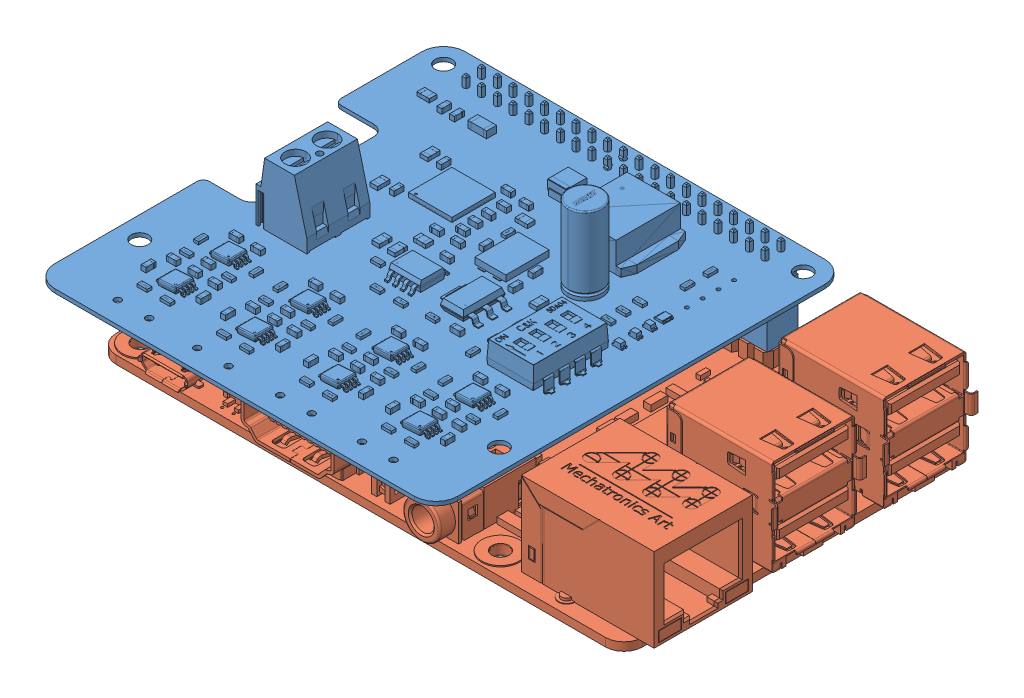
SolidWorks assembly pcbWithPi, configuration Default. Lengths in mm.
Overall size (89.64 32.52 66.38).
2 component instances, 2 part files, 3 mates.
Components (placement in the parent):
- Top-2: Top [Default] at (-4.2348 44.5064 41.2898) x (1 0 0) z (0 1 0) size (64.99 66.2 32.52)
- Raspberry Pi 3-2: Raspberry Pi 3 [Default] at (54.2115 28.8209 -21.0547) x (1 0 0) z (0 1 0) size (89.64 57.31 18.59)
Mates (geometry in assembly coordinates):
- Coincident1: coincident aligned: plane of Top-2 through (13.8195 46.2829 -48.7426) normal (-1 0 0); plane of Raspberry Pi 3-2 through (13.8195 32.3109 -49.3876) normal (-1 0 0)
- Coincident2: coincident aligned: plane of Top-2 through (13.8195 46.2829 -49.3776) normal (0 0 -1); plane of Raspberry Pi 3-2 through (14.4695 32.3109 -49.3776) normal (0 0 -1)
- Distance1: distance = 0.5 mm anti-aligned: plane of Top-2 through (63.921 32.8209 -47.7901) normal (0 -1 0); plane of Raspberry Pi 3-2 through (12.8595 32.3209 -45.4554) normal (0 1 0)
